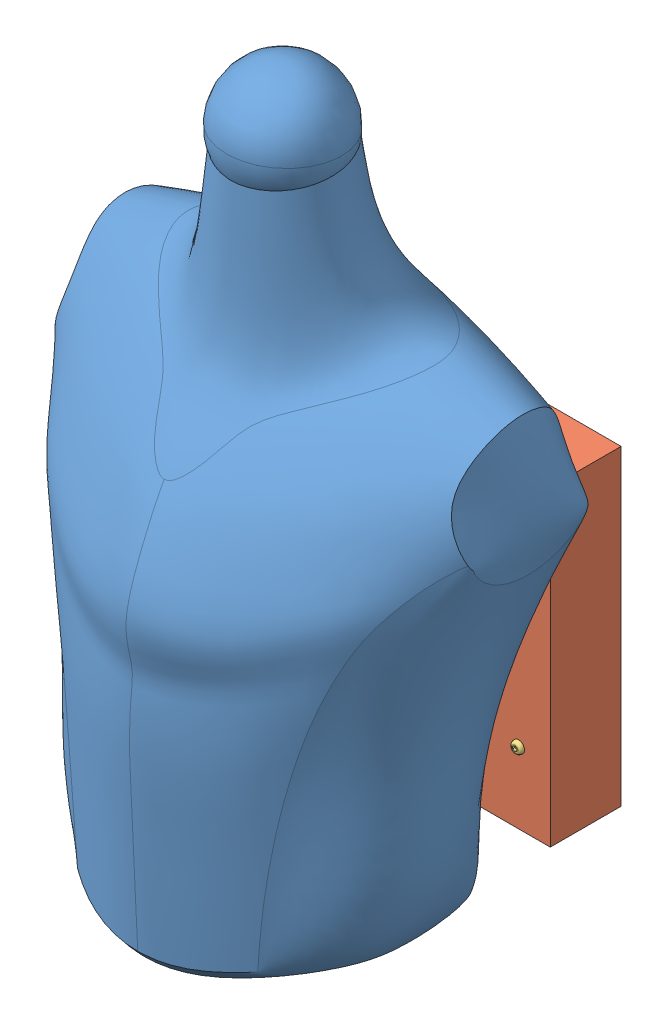
SolidWorks assembly ControlCircuitMount, configuration Default. Lengths in mm.
Overall size (402.84 950.58 367.01).
198 component instances, 41 part files, 56 mates.
Components (placement in the parent):
- AvgHumanBack-1: AvgHumanBack [Default] at origin size (402.84 950.58 279.6)
- ElectronicsBaseplate-1: ElectronicsBaseplate [Default] at (-35.085 1150.9976 -155.5) x (0 1 0) z (-1 0 0) size (224.52 47.62 183.13)
  - ControlPCB-1: ControlPCB [Default] at origin size (144.9 41.12 153.13)
    - MEGA2560+MotorShield-1: MEGA2560+MotorShield [Default] at origin size (108.32 25.5 53.3)
    - 1x2 Male Pin Header.step-1: 1x2 Male Pin Header.step [Default] at (-30.15 23.54 -23.8673) x (1 0 0) z (0 0 -1) size (5.08 13.54 2.5)
    - 1x6 Male Pin Header.step-1: 1x6 Male Pin Header.step [Default] at (-9.8 23.54 -23.8673) x (-1 0 0) z (0 0 1) size (15.24 13.54 2.5)
    - 1x5 Male Pin Header.step-1: 1x5 Male Pin Header.step [Default] at (-16.9 23.54 24.12) x (1 0 0) z (0 0 -1) size (12.71 13.54 2.5)
    - ADCPCB-1: ADCPCB [Default] at (-8.2861 23.54 0.0047) x (0.011416 0 0.999935) z (0 1 0) size (70.2 51.25 24.04)
      - 5x7PCBBoard.stp-1: 5x7PCBBoard.stp [Default] at origin size (70.2 50.2 1.66)
      - FemalePinHeader2By1.stp-1: FemalePinHeader2By1.stp [Default] at (-29.21 -21.59 1.54) x (0 1 0) z (0 0 1) size (5.08 2.54 11.7)
        - Female Pin Header 1x.stp-1: Female Pin Header 1x.stp [Default] at origin size (2.54 2.54 11.7)
        - Female Pin Header 1x.stp-2: Female Pin Header 1x.stp [Default] at (2.54 0 0) size (2.54 2.54 11.7)
      - FemalePinHeader2By1.stp-2: FemalePinHeader2By1.stp [Default] at (-29.21 -6.35 1.54) x (0 1 0) z (0 0 1) size (5.08 2.54 11.7)
        - Female Pin Header 1x.stp-1: Female Pin Header 1x.stp [Default] at origin size (2.54 2.54 11.7)
        - Female Pin Header 1x.stp-2: Female Pin Header 1x.stp [Default] at (2.54 0 0) size (2.54 2.54 11.7)
      - FemalePinHeader2By1.stp-3: FemalePinHeader2By1.stp [Default] at (-29.21 -19.05 1.54) x (0 1 0) z (0 0 1) size (5.08 2.54 11.7)
        - Female Pin Header 1x.stp-1: Female Pin Header 1x.stp [Default] at origin size (2.54 2.54 11.7)
        - Female Pin Header 1x.stp-2: Female Pin Header 1x.stp [Default] at (2.54 0 0) size (2.54 2.54 11.7)
      - FemalePinHeader2By1.stp-4: FemalePinHeader2By1.stp [Default] at (26.67 -21.59 1.54) x (0 1 0) z (0 0 1) size (5.08 2.54 11.7)
        - Female Pin Header 1x.stp-1: Female Pin Header 1x.stp [Default] at origin size (2.54 2.54 11.7)
        - Female Pin Header 1x.stp-2: Female Pin Header 1x.stp [Default] at (2.54 0 0) size (2.54 2.54 11.7)
      - FemalePinHeader2By1.stp-5: FemalePinHeader2By1.stp [Default] at (26.67 -19.05 1.54) x (0 1 0) z (0 0 1) size (5.08 2.54 11.7)
        - Female Pin Header 1x.stp-1: Female Pin Header 1x.stp [Default] at origin size (2.54 2.54 11.7)
        - Female Pin Header 1x.stp-2: Female Pin Header 1x.stp [Default] at (2.54 0 0) size (2.54 2.54 11.7)
      - FemalePinHeader10By1.stp-1: FemalePinHeader10By1.stp [Default] at (3.81 1.27 1.54) x (0 -1 0) z (0 0 1) size (25.4 2.54 11.7)
        - Female Pin Header 1x.stp-1: Female Pin Header 1x.stp [Default] at origin size (2.54 2.54 11.7)
        - Female Pin Header 1x.stp-2: Female Pin Header 1x.stp [Default] at (2.54 0 0) size (2.54 2.54 11.7)
        - Female Pin Header 1x.stp-3: Female Pin Header 1x.stp [Default] at (5.08 0 0) size (2.54 2.54 11.7)
        - Female Pin Header 1x.stp-4: Female Pin Header 1x.stp [Default] at (7.62 0 0) size (2.54 2.54 11.7)
        - Female Pin Header 1x.stp-5: Female Pin Header 1x.stp [Default] at (10.16 0 0) size (2.54 2.54 11.7)
        - Female Pin Header 1x.stp-6: Female Pin Header 1x.stp [Default] at (12.7 0 0) size (2.54 2.54 11.7)
        - Female Pin Header 1x.stp-7: Female Pin Header 1x.stp [Default] at (15.24 0 0) size (2.54 2.54 11.7)
        - Female Pin Header 1x.stp-8: Female Pin Header 1x.stp [Default] at (17.78 0 0) size (2.54 2.54 11.7)
        - Female Pin Header 1x.stp-9: Female Pin Header 1x.stp [Default] at (20.32 0 0) size (2.54 2.54 11.7)
        - Female Pin Header 1x.stp-10: Female Pin Header 1x.stp [Default] at (22.86 0 0) size (2.54 2.54 11.7)
      - FemalePinHeader6By1.stp-1: FemalePinHeader6By1.stp [Default] at (-13.97 21.59 1.54) x (0 -1 0) z (0 0 1) size (15.24 2.54 11.7)
        - Female Pin Header 1x.stp-1: Female Pin Header 1x.stp [Default] at origin size (2.54 2.54 11.7)
        - Female Pin Header 1x.stp-2: Female Pin Header 1x.stp [Default] at (2.54 0 0) size (2.54 2.54 11.7)
        - Female Pin Header 1x.stp-3: Female Pin Header 1x.stp [Default] at (5.08 0 0) size (2.54 2.54 11.7)
        - Female Pin Header 1x.stp-4: Female Pin Header 1x.stp [Default] at (7.62 0 0) size (2.54 2.54 11.7)
        - Female Pin Header 1x.stp-5: Female Pin Header 1x.stp [Default] at (10.16 0 0) size (2.54 2.54 11.7)
        - Female Pin Header 1x.stp-6: Female Pin Header 1x.stp [Default] at (12.7 0 0) size (2.54 2.54 11.7)
      - FemalePinHeader4By1.stp-1: FemalePinHeader4By1.stp [Default] at (11.44 19.05 1.54) x (0 -1 0) z (0 0 1) size (10.16 2.54 11.7)
        - Female Pin Header 1x.stp-1: Female Pin Header 1x.stp [Default] at origin size (2.54 2.54 11.7)
        - Female Pin Header 1x.stp-2: Female Pin Header 1x.stp [Default] at (2.54 0 0) size (2.54 2.54 11.7)
        - Female Pin Header 1x.stp-3: Female Pin Header 1x.stp [Default] at (5.08 0 0) size (2.54 2.54 11.7)
        - Female Pin Header 1x.stp-4: Female Pin Header 1x.stp [Default] at (7.62 0 0) size (2.54 2.54 11.7)
      - ADS1115+PinHeader.step-1: ADS1115+PinHeader.step [Default] at (144.065 -99.14 12.63) x (-1 0 0) z (0 0 1) size (17.14 27.94 11.54)
        - R_0805_2012Metric.step-1: R_0805_2012Metric.step [Default] at (149.225 -80.01 1.65) size (2 1.2 0.45)
          - SOLID.step-1: SOLID.step [Default] at origin size (2 1.2 0.45)
        - R_0805_2012Metric.step-2: R_0805_2012Metric.step [Default] at (149.225 -77.47 1.65) size (2 1.2 0.45)
          - SOLID.step-1: SOLID.step [Default] at origin size (2 1.2 0.45)
        - C_0603_1608Metric.step-1: C_0603_1608Metric.step [Default] at (150.495 -96.52 1.65) x (0 1 0) z (0 0 1) size (1.6 0.8 0.8)
          - SOLID-0.step-1: SOLID-0.step [Default] at origin size (1.6 0.8 0.8)
        - TSSOP-10_3x3mm_P0.5mm.step-1: TSSOP-10_3x3mm_P0.5mm.step [Default] at (147.32 -96.52 1.65) x (0 -1 0) z (0 0 1) size (4.9 3 1)
          - SOLID-1.step-1: SOLID-1.step [Default] at origin size (4.9 3 1)
        - PinHeader_1x10_P2.54mm_Vertical.step-1: PinHeader_1x10_P2.54mm_Vertical.step [Default] at (140.335 -77.47 -0.05) x (-1 0 0) z (0 0 -1) size (2.54 25.4 11.54)
          - SOLID-2.step-1: SOLID-2.step [Default] at origin size (2.54 25.4 11.54)
        - C_0603_1608Metric.step-2: C_0603_1608Metric.step [Default] at (146.05 -78.74 1.65) x (0 1 0) z (0 0 1) size (1.6 0.8 0.8)
          - SOLID-0.step-1: SOLID-0.step [Default] at origin size (1.6 0.8 0.8)
        - R_0402_1005Metric.step-1: R_0402_1005Metric.step [Default] at (149.225 -85.09 1.65) x (-1 0 0) z (0 0 1) size (1 0.5 0.35)
          - SOLID-3.step-1: SOLID-3.step [Default] at origin size (1 0.5 0.35)
        - R_0402_1005Metric.step-2: R_0402_1005Metric.step [Default] at (149.225 -82.55 1.65) x (-1 0 0) z (0 0 1) size (1 0.5 0.35)
          - SOLID-3.step-1: SOLID-3.step [Default] at origin size (1 0.5 0.35)
        - R_0402_1005Metric.step-3: R_0402_1005Metric.step [Default] at (149.225 -87.63 1.65) size (1 0.5 0.35)
          - SOLID-3.step-1: SOLID-3.step [Default] at origin size (1 0.5 0.35)
        - R_0402_1005Metric.step-4: R_0402_1005Metric.step [Default] at (149.225 -90.17 1.65) x (-1 0 0) z (0 0 1) size (1 0.5 0.35)
          - SOLID-3.step-1: SOLID-3.step [Default] at origin size (1 0.5 0.35)
        - COMPOUND.step-1: COMPOUND.step [Default] at origin size (17.14 27.94 1.6)
      - 1x4 Male Pin Header.step-1: 1x4 Male Pin Header.step [Default] at (11.52 11.51 12.58) x (0 1 0) z (-1 0 0) size (10.17 13.54 2.5)
      - 1x6 Male Pin Header.step-1: 1x6 Male Pin Header.step [Default] at (-13.89 8.97 12.58) x (0 1 0) z (-1 0 0) size (15.24 13.54 2.5)
      - HX711.STEP-1: HX711.STEP [Default] at (-17.9207 5.1545 12.58) size (34 21 1.97)
        - HX711_SOP16_Valor predeterminado.STEP-1: HX711_SOP16_Valor predeterminado.STEP [Default] at (16.3915 14.4374 -9.5535) size (6.7 10 1.56)
          - base_HX711_Valor predeterminado.STEP-1: base_HX711_Valor predeterminado.STEP [Default] at (0.6189 -0.8581 10) size (4.4 10 1.52)
          - pino_HX711_Valor predeterminado.STEP-1: pino_HX711_Valor predeterminado.STEP [Default] at (-2.7311 3.5869 10.04) x (0 -1 0) z (-1 0 0) size (0.4 0.86 1.3)
          - pino_HX711_Valor predeterminado.STEP-2: pino_HX711_Valor predeterminado.STEP [Default] at (-2.7311 2.3169 10.04) x (0 -1 0) z (-1 0 0) size (0.4 0.86 1.3)
          - pino_HX711_Valor predeterminado.STEP-3: pino_HX711_Valor predeterminado.STEP [Default] at (-2.7311 1.0469 10.04) x (0 -1 0) z (-1 0 0) size (0.4 0.86 1.3)
          - pino_HX711_Valor predeterminado.STEP-4: pino_HX711_Valor predeterminado.STEP [Default] at (-2.7311 -0.2231 10.04) x (0 -1 0) z (-1 0 0) size (0.4 0.86 1.3)
          - pino_HX711_Valor predeterminado.STEP-5: pino_HX711_Valor predeterminado.STEP [Default] at (-2.7311 -1.4931 10.04) x (0 -1 0) z (-1 0 0) size (0.4 0.86 1.3)
          - pino_HX711_Valor predeterminado.STEP-6: pino_HX711_Valor predeterminado.STEP [Default] at (-2.7311 -2.7631 10.04) x (0 -1 0) z (-1 0 0) size (0.4 0.86 1.3)
          - pino_HX711_Valor predeterminado.STEP-7: pino_HX711_Valor predeterminado.STEP [Default] at (-2.7311 -4.0331 10.04) x (0 -1 0) z (-1 0 0) size (0.4 0.86 1.3)
          - pino_HX711_Valor predeterminado.STEP-8: pino_HX711_Valor predeterminado.STEP [Default] at (-2.7311 -5.3031 10.04) x (0 -1 0) z (-1 0 0) size (0.4 0.86 1.3)
          - pino_HX711_Valor predeterminado.STEP-9: pino_HX711_Valor predeterminado.STEP [Default] at (3.9689 3.5869 10.04) x (0 1 0) z (1 0 0) size (0.4 0.86 1.3)
          - pino_HX711_Valor predeterminado.STEP-10: pino_HX711_Valor predeterminado.STEP [Default] at (3.9689 2.3169 10.04) x (0 1 0) z (1 0 0) size (0.4 0.86 1.3)
          - pino_HX711_Valor predeterminado.STEP-11: pino_HX711_Valor predeterminado.STEP [Default] at (3.9689 1.0469 10.04) x (0 1 0) z (1 0 0) size (0.4 0.86 1.3)
          - pino_HX711_Valor predeterminado.STEP-12: pino_HX711_Valor predeterminado.STEP [Default] at (3.9689 -0.2231 10.04) x (0 1 0) z (1 0 0) size (0.4 0.86 1.3)
          - pino_HX711_Valor predeterminado.STEP-13: pino_HX711_Valor predeterminado.STEP [Default] at (3.9689 -1.4931 10.04) x (0 1 0) z (1 0 0) size (0.4 0.86 1.3)
          - pino_HX711_Valor predeterminado.STEP-14: pino_HX711_Valor predeterminado.STEP [Default] at (3.9689 -2.7631 10.04) x (0 1 0) z (1 0 0) size (0.4 0.86 1.3)
          - pino_HX711_Valor predeterminado.STEP-15: pino_HX711_Valor predeterminado.STEP [Default] at (3.9689 -4.0331 10.04) x (0 1 0) z (1 0 0) size (0.4 0.86 1.3)
          - pino_HX711_Valor predeterminado.STEP-16: pino_HX711_Valor predeterminado.STEP [Default] at (3.9689 -5.3031 10.04) x (0 1 0) z (1 0 0) size (0.4 0.86 1.3)
        - SOT23_Valor predeterminado.STEP-1: SOT23_Valor predeterminado.STEP [Default] at (9.1544 19.1355 -2.4535) x (-1 0 0) z (0 0 1) size (2.3 2.9 1.03)
          - TRANSISTOR_SOT23_Valor predeterminado.STEP-1: TRANSISTOR_SOT23_Valor predeterminado.STEP [Default] at (0.0204 0.1428 2.9) size (1.3 2.9 1)
          - PINO_SOT23_Valor predeterminado.STEP-1: PINO_SOT23_Valor predeterminado.STEP [Default] at (-1.1296 1.0928 2.94) x (0 -1 0) z (-1 0 0) size (0.4 0.61 0.65)
          - PINO_SOT23_Valor predeterminado.STEP-2: PINO_SOT23_Valor predeterminado.STEP [Default] at (-1.1296 -0.8072 2.94) x (0 -1 0) z (-1 0 0) size (0.4 0.61 0.65)
          - PINO_SOT23_Valor predeterminado.STEP-3: PINO_SOT23_Valor predeterminado.STEP [Default] at (1.1704 0.1428 2.94) x (0 1 0) z (1 0 0) size (0.4 0.61 0.65)
        - placa_Valor predeterminado.STEP-1: placa_Valor predeterminado.STEP [Default] at origin size (34 21 0.41)
        - RESISTOR_SMD_122_Valor predeterminado.STEP-1: RESISTOR_SMD_122_Valor predeterminado.STEP [Default] at (7.557 7.2289 0.4215) x (0 1 0) z (-1 0 0) size (2 0.82 1.27)
        - RESISTOR_SMD_122_Valor predeterminado.STEP-2: RESISTOR_SMD_122_Valor predeterminado.STEP [Default] at (26.4556 7.0756 0.4215) x (0 1 0) z (-1 0 0) size (2 0.82 1.27)
        - RESISTOR_SMD_822_Valor predeterminado.STEP-1: RESISTOR_SMD_822_Valor predeterminado.STEP [Default] at (8.9272 12.9039 0.4215) x (-1 0 0) z (0 -1 0) size (2 0.82 1.27)
        - RESISTOR_SMD_203_Valor predeterminado.STEP-1: RESISTOR_SMD_203_Valor predeterminado.STEP [Default] at (8.9446 15.4759 0.4215) x (-1 0 0) z (0 -1 0) size (2 0.82 1.27)
        - CAPACITOR_805_Valor predeterminado.STEP-1: CAPACITOR_805_Valor predeterminado.STEP [Default] at (14.517 4.7561 0.4215) x (1 0 0) z (0 1 0) size (2 0.8 1.27)
        - CAPACITOR_805_Valor predeterminado.STEP-2: CAPACITOR_805_Valor predeterminado.STEP [Default] at (24.8147 18.1011 0.4215) x (1 0 0) z (0 1 0) size (2 0.8 1.27)
        - CAPACITOR_805_Valor predeterminado.STEP-3: CAPACITOR_805_Valor predeterminado.STEP [Default] at (19.4533 4.8571 0.4215) x (1 0 0) z (0 1 0) size (2 0.8 1.27)
        - CAPACITOR_805_Valor predeterminado.STEP-4: CAPACITOR_805_Valor predeterminado.STEP [Default] at (23.7861 6.9684 0.4215) x (0 -1 0) z (1 0 0) size (2 0.8 1.27)
        - CAPACITOR_805_Valor predeterminado.STEP-5: CAPACITOR_805_Valor predeterminado.STEP [Default] at (10.279 7.2922 0.4215) x (0 -1 0) z (1 0 0) size (2 0.8 1.27)
      - 1x2 Male Pin Header.step-1: 1x2 Male Pin Header.step [Default] at (-29.29 -19.13 10.04) x (0 -1 0) z (-1 0 0) size (5.08 13.54 2.5) (hidden)
      - 1x2 Male Pin Header.step-2: 1x2 Male Pin Header.step [Default] at (-29.29 -3.89 10.04) x (0 -1 0) z (-1 0 0) size (5.08 13.54 2.5) (hidden)
      - 1x2 Male Pin Header.step-3: 1x2 Male Pin Header.step [Default] at (26.59 -16.59 10.04) x (0 -1 0) z (-1 0 0) size (5.08 13.54 2.5) (hidden)
      - 5mm2PTerminalBlock-1: 5mm2PTerminalBlock [Default] at (-25.19 24.09 1.54) x (0 -1 0) z (0 0 1) size (10.6 7.6 15)
      - 5mm2PTerminalBlock-2: 5mm2PTerminalBlock [Default] at (-25.19 13.89 1.54) x (0 -1 0) z (0 0 1) size (10.6 7.6 15)
      - 5mm2PTerminalBlock-3: 5mm2PTerminalBlock [Default] at (3.69 25.19 1.54) x (-1 0 0) z (0 0 1) size (10.6 7.6 15)
      - 5mm2PTerminalBlock-4: 5mm2PTerminalBlock [Default] at (15.04 -6.23 1.54) x (0 1 0) z (0 0 1) size (10.6 7.6 15)
    - BLEShuntPCB-1: BLEShuntPCB [Default] at (-12.5947 21 -49.5125) x (-1 0 0) z (0 -1 0) size (73.24 30.62 25.87)
      - 3x7PerfBoard-1: 3x7PerfBoard [Default] at origin size (70.1 30.1 1.65)
      - 5mm2PTerminalBlock-1: 5mm2PTerminalBlock [Default] at (-19.17 15.03 1.55) x (-1 0 0) z (0 0 1) size (10.6 7.6 15)
      - FemalePinHeader8By1.stp-1: FemalePinHeader8By1.stp [Default] at (-16.51 6.35 1.55) x (0 -1 0) z (0 0 1) size (20.32 2.54 11.7)
        - Female Pin Header 1x.stp-1: Female Pin Header 1x.stp [Default] at origin size (2.54 2.54 11.7)
        - Female Pin Header 1x.stp-2: Female Pin Header 1x.stp [Default] at (2.54 0 0) size (2.54 2.54 11.7)
        - Female Pin Header 1x.stp-3: Female Pin Header 1x.stp [Default] at (5.08 0 0) size (2.54 2.54 11.7)
        - Female Pin Header 1x.stp-4: Female Pin Header 1x.stp [Default] at (7.62 0 0) size (2.54 2.54 11.7)
        - Female Pin Header 1x.stp-5: Female Pin Header 1x.stp [Default] at (10.16 0 0) size (2.54 2.54 11.7)
        - Female Pin Header 1x.stp-6: Female Pin Header 1x.stp [Default] at (12.7 0 0) size (2.54 2.54 11.7)
        - Female Pin Header 1x.stp-7: Female Pin Header 1x.stp [Default] at (15.24 0 0) size (2.54 2.54 11.7)
        - Female Pin Header 1x.stp-8: Female Pin Header 1x.stp [Default] at (17.78 0 0) size (2.54 2.54 11.7)
      - 1x8 Male Pin Header.step-1: 1x8 Male Pin Header.step [Default] at (-16.59 6.27 12.59) x (0 -1 0) z (1 0 0) size (20.32 13.54 2.5)
      - BLEFriend.stp-1: BLEFriend.stp [Default] at (-19.31 8.128 12.59) x (0 -1 0) z (0 0 1) size (21.35 31.87 4.78)
      - 5mm2PTerminalBlock-2: 5mm2PTerminalBlock [Default] at (24.01 15.03 1.55) x (-1 0 0) z (0 0 1) size (10.6 7.6 15)
      - 5mm2PTerminalBlock-5: 5mm2PTerminalBlock [Default] at (14.1 -15.03 1.55) size (10.6 7.6 15)
      - FemalePinHeader2By1-1: FemalePinHeader2By1 [Default] at (-29.21 -8.89 0) x (0 -1 0) z (0 0 -1) size (5.08 2.54 11.7)
      - FemalePinHeader2By1-2: FemalePinHeader2By1 [Default] at (-29.21 6.35 0) x (0 -1 0) z (0 0 -1) size (5.08 2.54 11.7)
      - FemalePinHeader2By1-3: FemalePinHeader2By1 [Default] at (26.67 -6.35 0) x (0 -1 0) z (0 0 -1) size (5.08 2.54 11.7)
      - ShuntResistor-1: ShuntResistor [Default<As Machined>] at (18.3281 0.2483 1.55) x (0.946299 -0.323291 0) z (-0.323291 -0.946299 0) size (35 9.71 20.4)
    - RelayPCB-1: RelayPCB [Default] at (46.44 18.5 -16.8) x (0 0 -1) z (1 0 0) size (51 20.5 20)
    - ThermistorPCB-1: ThermistorPCB [Default] at (53.61 18 26.48) x (0 0 -1) z (1 0 0) size (30 20 70)
    - RelayPCB-2: RelayPCB [Default] at (109.78 0 -53.12) size (55.5 16.25 117.54)
      - 4-Port Relay-1: 4-Port Relay [Default] at origin size (55.5 16.25 75.54)
      - 2-Port Relay-1: 2-Port Relay [Default] at (2.75 0 60.27) size (50 16.25 39)
    - LM2596-BuckConverter-1: LM2596-BuckConverter [Default] at (-16.99 0 -92.15) x (-1 0 0) z (0 1 0) size (65 39 13)
    - LM2596-BuckConverter-2: LM2596-BuckConverter [Default] at (48.77 0 -79.15) x (0 0 -1) z (0 1 0) size (65 39 13)
  - Baseplate^ElectronicsBaseplate-1: Baseplate^ElectronicsBaseplate [Default] at (30 0 0) size (224.52 14.95 183.13) (virtual)
  - M3x8-1: M3x8 [Default] at (-35.49 -5.5 24.11) x (1 0 0) z (0 -1 0) size (5.5 5.5 11)
  - M3x8-2: M3x8 [Default] at (46.98 -5.5 24.11) x (1 0 0) z (0 -1 0) size (5.5 5.5 11)
  - M3x8-3: M3x8 [Default] at (40.62 -5.5 -24.11) x (1 0 0) z (0 -1 0) size (5.5 5.5 11)
  - M3x8-4: M3x8 [Default] at (-34.26 -5.5 -24.11) x (1 0 0) z (0 -1 0) size (5.5 5.5 11)
  - M3x8-5: M3x8 [Default] at (-45.99 -5.5 -76.15) x (1 0 0) z (0 -1 0) size (5.5 5.5 11)
  - M3x8-6: M3x8 [Default] at (12.01 -5.5 -76.15) x (1 0 0) z (0 -1 0) size (5.5 5.5 11)
  - M3x8-7: M3x8 [Default] at (-45.99 -5.5 -108.15) x (1 0 0) z (0 -1 0) size (5.5 5.5 11)
  - M3x8-8: M3x8 [Default] at (12.01 -5.5 -108.15) x (1 0 0) z (0 -1 0) size (5.5 5.5 11)
  - M3x8-9: M3x8 [Default] at (32.77 -5.5 -50.15) x (1 0 0) z (0 -1 0) size (5.5 5.5 11)
  - M3x8-10: M3x8 [Default] at (64.77 -5.5 -50.15) x (1 0 0) z (0 -1 0) size (5.5 5.5 11)
  - M3x8-11: M3x8 [Default] at (32.77 -5.5 -108.15) x (1 0 0) z (0 -1 0) size (5.5 5.5 11)
  - M3x8-12: M3x8 [Default] at (64.77 -5.5 -108.15) x (1 0 0) z (0 -1 0) size (5.5 5.5 11)
  - M3x8-13: M3x8 [Default] at (85.655 -5.5 -87.245) x (1 0 0) z (0 -1 0) size (5.5 5.5 11)
  - M3x8-14: M3x8 [Default] at (133.905 -5.5 -87.245) x (1 0 0) z (0 -1 0) size (5.5 5.5 11)
  - M3x8-15: M3x8 [Default] at (133.905 -5.5 -18.995) x (1 0 0) z (0 -1 0) size (5.5 5.5 11)
  - M3x8-16: M3x8 [Default] at (85.655 -5.5 -18.995) x (1 0 0) z (0 -1 0) size (5.5 5.5 11)
  - M3x8-17: M3x8 [Default] at (89.905 -5.5 -9.6) x (1 0 0) z (0 -1 0) size (5.5 5.5 11)
  - M3x8-18: M3x8 [Default] at (135.155 -5.5 -9.6) x (1 0 0) z (0 -1 0) size (5.5 5.5 11)
  - M3x8-19: M3x8 [Default] at (89.905 -5.5 23.9) x (1 0 0) z (0 -1 0) size (5.5 5.5 11)
  - M3x8-20: M3x8 [Default] at (135.155 -5.5 23.9) x (1 0 0) z (0 -1 0) size (5.5 5.5 11)
  - M3x8-22: M3x8 [Default] at (16.53 -5.5 -8.88) x (1 0 0) z (0 -1 0) size (5.5 5.5 11)
  - M3x8-23: M3x8 [Default] at (16.53 -5.5 19.03) x (1 0 0) z (0 -1 0) size (5.5 5.5 11)
  - M3Nut-1: M3Nut [Default] at (32.77 1.5 -108.15) size (6 2.34 5.2)
  - M3Nut-2: M3Nut [Default] at (64.77 1.5 -108.15) size (6 2.34 5.2)
  - M3Nut-3: M3Nut [Default] at (32.77 1.5 -50.15) size (6 2.34 5.2)
  - M3Nut-4: M3Nut [Default] at (64.77 1.5 -50.15) size (6 2.34 5.2)
  - M3Nut-7: M3Nut [Default] at (12.01 1.5 -108.15) size (6 2.34 5.2)
  - M3Nut-8: M3Nut [Default] at (-45.99 1.5 -108.15) size (6 2.34 5.2)
  - M3Nut-9: M3Nut [Default] at (-45.99 1.5 -76.15) size (6 2.34 5.2)
  - M3Nut-10: M3Nut [Default] at (12.01 1.5 -76.15) size (6 2.34 5.2)
  - M3Nut-11: M3Nut [Default] at (-34.26 1.5 -24.11) size (6 2.34 5.2)
  - M3Nut-12: M3Nut [Default] at (-35.49 1.5 24.11) size (6 2.34 5.2)
  - M3Nut-13: M3Nut [Default] at (16.53 1.5 19.03) size (6 2.34 5.2)
  - M3Nut-14: M3Nut [Default] at (16.53 1.5 -8.88) size (6 2.34 5.2)
  - M3Nut-17: M3Nut [Default] at (85.655 1.75 -87.245) size (6 2.34 5.2)
  - M3Nut-19: M3Nut [Default] at (133.905 1.75 -87.245) size (6 2.34 5.2)
  - M3Nut-20: M3Nut [Default] at (133.905 1.75 -18.995) size (6 2.34 5.2)
  - M3Nut-21: M3Nut [Default] at (85.655 1.75 -18.995) size (6 2.34 5.2)
  - M3Nut-22: M3Nut [Default] at (89.905 1.75 -9.6) size (6 2.34 5.2)
  - M3Nut-23: M3Nut [Default] at (135.155 1.75 -9.6) size (6 2.34 5.2)
  - M3Nut-24: M3Nut [Default] at (135.155 1.75 23.9) size (6 2.34 5.2)
  - M3Nut-25: M3Nut [Default] at (89.905 1.75 23.9) size (6 2.34 5.2)
- PlasticBox-1: PlasticBox [Default] at (11.048 1111.6872 -147) size (215.9 279.4 63.5)
- M6x12_Buttonhead-1: M6x12_Buttonhead [Default] at (83.565 1203.7676 -144) x (0.866025 0.5 0) z (0 0 1) size (10.53 10.53 15.3)
- M6x12_Buttonhead-2: M6x12_Buttonhead [Default] at (49.565 1296.0276 -144) x (0.866025 0.5 0) z (0 0 1) size (10.53 10.53 15.3)
- M6x12_Buttonhead-3: M6x12_Buttonhead [Default] at (79.565 1093.5076 -144) x (0.866025 0.5 0) z (0 0 1) size (10.53 10.53 15.3)
- M6x12_Buttonhead-4: M6x12_Buttonhead [Default] at (-79.565 1296.0276 -144) x (0.866025 0.5 0) z (0 0 1) size (10.53 10.53 15.3)
- M6x12_Buttonhead-5: M6x12_Buttonhead [Default] at (-79.565 1203.7676 -144) x (0.866025 0.5 0) z (0 0 1) size (10.53 10.53 15.3)
- M6x12_Buttonhead-6: M6x12_Buttonhead [Default] at (-79.565 1093.5076 -144) x (0.866025 0.5 0) z (0 0 1) size (10.53 10.53 15.3)
- M6Nut-1: M6Nut [Default] at (79.565 1093.5076 -153) x (0 1 0) z (-1 0 0) size (11.08 5.03 10.65)
- M6Nut-2: M6Nut [Default] at (83.565 1203.7676 -153) x (0 1 0) z (-1 0 0) size (11.08 5.03 10.65)
- M6Nut-3: M6Nut [Default] at (49.565 1296.0276 -153) x (0 1 0) z (-1 0 0) size (11.08 5.03 10.65)
- M6Nut-4: M6Nut [Default] at (-79.565 1296.0276 -153) x (0 1 0) z (-1 0 0) size (11.08 5.03 10.65)
- M6Nut-5: M6Nut [Default] at (-79.565 1203.7676 -153) x (0 1 0) z (-1 0 0) size (11.08 5.03 10.65)
- M6Nut-6: M6Nut [Default] at (-79.565 1093.5076 -153) x (0 1 0) z (-1 0 0) size (11.08 5.03 10.65)
- BatteryMount-1: BatteryMount [Default] at (42.2 1067.9476 -164.44) x (1 0 0) z (0 1 0) size (166.9 85.99 60.11)
  - BatteryPack-1: BatteryPack [Default] at origin size (166.9 85.99 36.23)
  - BatteryPack-2: BatteryPack [Default] at (0 0 -23.88) size (166.9 85.99 36.23)
Mates (geometry in assembly coordinates):
- Coincident1: coincident aligned: plane of AvgHumanBack-1 through (0 0 0) normal (0 0 1)
- Coincident2: coincident aligned: plane of AvgHumanBack-1 through (0 0 0) normal (0 1 0)
- Coincident3: coincident aligned: plane of AvgHumanBack-1 through (0 0 0) normal (1 0 0)
- Parallel1: parallel aligned: plane of ElectronicsBaseplate-1/Baseplate^ElectronicsBaseplate-1 through (-35.085 1180.9976 -150) normal (0 0 1)
- Coincident6: coincident aligned: plane of ElectronicsBaseplate-1/Baseplate^ElectronicsBaseplate-1 through (-35.085 1180.9976 -150) normal (0 0 1)
- Tangent1: tangent: face of ?; plane of assembly through (0 0 -150) normal (0 0 1)
- Symmetric2: symmetric aligned: plane of BatteryPack-1 through (66.3 1055.1849 -161.49) normal (1 0 0); plane of BatteryPack-1 through (-66.3 1055.1849 -161.49) normal (-1 0 0)
- InPlace1: in place: plane of AvgHumanBack-1 through (0 0 0) normal (0 0 1); moOrthogonalPlaneRef_w of AvgHumanBack-1 through (0 0 0) normal (0 1 0); plane of AvgHumanBack-1 through (0 0 0) normal (1 0 0); unknown of AvgHumanBack-1
- Coincident10: coincident aligned: 
- Coincident11: coincident aligned: plane of Part1^ControlCircuitMount-1 through (0 0 0) normal (0 1 0)
- Coincident12: coincident anti-aligned: plane of Part1^ControlCircuitMount-1 through (0 0 0) normal (1 0 0)
- Symmetric5: symmetric aligned: plane of Tote^ControlCircuitMount-1 through (104.95 1032.6276 -207.5) normal (-1 0 0); plane of Tote^ControlCircuitMount-1 through (-104.95 1306.0276 -207.5) normal (1 0 0)
- Coincident26: coincident anti-aligned: plane of ElectronicsBaseplate-1/M3x8-3 through (-10.975 1191.6176 -147) normal (0 0 1); plane of Tote^ControlCircuitMount-1 through (11.048 1111.6872 -147) normal (0 0 -1)
- Coincident17: coincident: point of AvgHumanBack-1; plane of Tote^ControlCircuitMount-1 through (-107.95 1029.6276 -144) normal (0 -1 0)
- Coincident18: coincident anti-aligned: plane of Tote^ControlCircuitMount-1 through (11.048 1111.6872 -144) normal (0 0 1); plane of M6x12_Buttonhead-1 through (83.565 1203.7676 -144) normal (0 0 -1)
- Parallel3: parallel anti-aligned: plane of Tote^ControlCircuitMount-1 through (-107.95 1309.0276 -144) normal (-1 0 0); plane of M6x12_Buttonhead-1 through (81.5645 1204.9226 -142.78) normal (1 0 0)
- Concentric1: concentric aligned: circle of Tote^ControlCircuitMount-1; circle of M6x12_Buttonhead-1
- Coincident20: coincident anti-aligned: plane of Tote^ControlCircuitMount-1 through (11.048 1111.6872 -144) normal (0 0 1); plane of M6x12_Buttonhead-2 through (49.565 1296.0276 -144) normal (0 0 -1)
- Parallel4: parallel anti-aligned: plane of Tote^ControlCircuitMount-1 through (-107.95 1309.0276 -144) normal (-1 0 0); plane of M6x12_Buttonhead-2 through (47.5645 1297.1826 -142.78) normal (1 0 0)
- Concentric2: concentric aligned: circle of Tote^ControlCircuitMount-1; circle of M6x12_Buttonhead-2
- Coincident21: coincident anti-aligned: plane of Tote^ControlCircuitMount-1 through (11.048 1111.6872 -144) normal (0 0 1); plane of M6x12_Buttonhead-3 through (79.565 1093.5076 -144) normal (0 0 -1)
- Parallel5: parallel anti-aligned: plane of Tote^ControlCircuitMount-1 through (-107.95 1309.0276 -144) normal (-1 0 0); plane of M6x12_Buttonhead-3 through (77.5645 1094.6626 -142.78) normal (1 0 0)
- Concentric3: concentric aligned: circle of Tote^ControlCircuitMount-1; circle of M6x12_Buttonhead-3
- Coincident22: coincident anti-aligned: plane of Tote^ControlCircuitMount-1 through (11.048 1111.6872 -144) normal (0 0 1); plane of M6x12_Buttonhead-4 through (-79.565 1296.0276 -144) normal (0 0 -1)
- Parallel6: parallel anti-aligned: plane of Tote^ControlCircuitMount-1 through (-107.95 1309.0276 -144) normal (-1 0 0); plane of M6x12_Buttonhead-4 through (-81.5655 1297.1826 -142.78) normal (1 0 0)
- Concentric4: concentric aligned: circle of Tote^ControlCircuitMount-1; circle of M6x12_Buttonhead-4
- Coincident23: coincident anti-aligned: plane of Tote^ControlCircuitMount-1 through (11.048 1111.6872 -144) normal (0 0 1); plane of M6x12_Buttonhead-5 through (-79.565 1203.7676 -144) normal (0 0 -1)
- Parallel7: parallel anti-aligned: plane of Tote^ControlCircuitMount-1 through (-107.95 1309.0276 -144) normal (-1 0 0); plane of M6x12_Buttonhead-5 through (-81.5655 1204.9226 -142.78) normal (1 0 0)
- Concentric5: concentric aligned: circle of Tote^ControlCircuitMount-1; circle of M6x12_Buttonhead-5
- Coincident24: coincident anti-aligned: plane of Tote^ControlCircuitMount-1 through (11.048 1111.6872 -144) normal (0 0 1); plane of M6x12_Buttonhead-6 through (-79.565 1093.5076 -144) normal (0 0 -1)
- Parallel8: parallel anti-aligned: plane of Tote^ControlCircuitMount-1 through (-107.95 1309.0276 -144) normal (-1 0 0); plane of M6x12_Buttonhead-6 through (-81.5655 1094.6626 -142.78) normal (1 0 0)
- Parallel10: parallel anti-aligned: plane of Tote^ControlCircuitMount-1 through (104.95 1032.6276 -207.5) normal (-1 0 0); plane of M6Nut-1 through (84.49 1096.351 -157.85) normal (1 0 0)
- Concentric7: concentric aligned: circle of M6x12_Buttonhead-3; circle of M6Nut-1
- Parallel11: parallel anti-aligned: plane of Tote^ControlCircuitMount-1 through (104.95 1032.6276 -207.5) normal (-1 0 0); plane of M6Nut-2 through (88.49 1206.611 -157.85) normal (1 0 0)
- Concentric8: concentric aligned: circle of M6x12_Buttonhead-1; circle of M6Nut-2
- Parallel12: parallel anti-aligned: plane of Tote^ControlCircuitMount-1 through (104.95 1032.6276 -207.5) normal (-1 0 0); plane of M6Nut-3 through (54.49 1298.871 -157.85) normal (1 0 0)
- Concentric9: concentric aligned: circle of M6x12_Buttonhead-2; circle of M6Nut-3
- Parallel13: parallel anti-aligned: plane of Tote^ControlCircuitMount-1 through (104.95 1032.6276 -207.5) normal (-1 0 0); plane of M6Nut-4 through (-74.64 1298.871 -157.85) normal (1 0 0)
- Concentric10: concentric aligned: circle of M6x12_Buttonhead-4; circle of M6Nut-4
- Parallel14: parallel anti-aligned: plane of Tote^ControlCircuitMount-1 through (104.95 1032.6276 -207.5) normal (-1 0 0); plane of M6Nut-5 through (-74.64 1206.611 -157.85) normal (1 0 0)
- Concentric11: concentric aligned: circle of M6x12_Buttonhead-5; circle of M6Nut-5
- Parallel15: parallel anti-aligned: plane of Tote^ControlCircuitMount-1 through (104.95 1032.6276 -207.5) normal (-1 0 0); plane of M6Nut-6 through (-74.64 1096.351 -157.85) normal (1 0 0)
- Concentric12: concentric aligned: circle of M6x12_Buttonhead-6; circle of M6Nut-6
- Parallel16: parallel anti-aligned: plane of ElectronicsBaseplate-1/Baseplate^ElectronicsBaseplate-1 through (-91.565 1081.5076 -150) normal (0 -1 0); plane of Tote^ControlCircuitMount-1 through (-104.95 1032.6276 -207.5) normal (0 1 0)
- Symmetric6: symmetric aligned: plane of ElectronicsBaseplate-1/Baseplate^ElectronicsBaseplate-1 through (-91.565 1306.0276 -150) normal (-1 0 0); plane of ElectronicsBaseplate-1/Baseplate^ElectronicsBaseplate-1 through (91.565 1081.5076 -150) normal (1 0 0)
- Coincident36: coincident anti-aligned: plane of ElectronicsBaseplate-1/Baseplate^ElectronicsBaseplate-1 through (61.565 1306.0276 -150) normal (0 1 0); plane of Tote^ControlCircuitMount-1 through (104.95 1306.0276 -207.5) normal (0 -1 0)
- Concentric13: concentric anti-aligned: circle of ElectronicsBaseplate-1/Baseplate^ElectronicsBaseplate-1; circle of M6x12_Buttonhead-6
- Coincident37: coincident anti-aligned: plane of ElectronicsBaseplate-1/Baseplate^ElectronicsBaseplate-1 through (-35.085 1180.9976 -153) normal (0 0 -1); plane of M6Nut-1 through (79.565 1093.5076 -153) normal (0 0 1)
- Coincident38: coincident anti-aligned: plane of ElectronicsBaseplate-1/Baseplate^ElectronicsBaseplate-1 through (-35.085 1180.9976 -153) normal (0 0 -1); plane of M6Nut-6 through (-79.565 1093.5076 -153) normal (0 0 1)
- Coincident39: coincident anti-aligned: plane of ElectronicsBaseplate-1/Baseplate^ElectronicsBaseplate-1 through (-35.085 1180.9976 -153) normal (0 0 -1); plane of M6Nut-5 through (-79.565 1203.7676 -153) normal (0 0 1)
- Coincident40: coincident anti-aligned: plane of ElectronicsBaseplate-1/Baseplate^ElectronicsBaseplate-1 through (-35.085 1180.9976 -153) normal (0 0 -1); plane of M6Nut-2 through (83.565 1203.7676 -153) normal (0 0 1)
- Coincident41: coincident anti-aligned: plane of ElectronicsBaseplate-1/Baseplate^ElectronicsBaseplate-1 through (-35.085 1180.9976 -153) normal (0 0 -1); plane of M6Nut-4 through (-79.565 1296.0276 -153) normal (0 0 1)
- Coincident42: coincident anti-aligned: plane of ElectronicsBaseplate-1/Baseplate^ElectronicsBaseplate-1 through (-35.085 1180.9976 -153) normal (0 0 -1); plane of M6Nut-3 through (49.565 1296.0276 -153) normal (0 0 1)
- Symmetric7: symmetric aligned: plane of BatteryMount-1/BatteryPack-2 through (66.3 1044.0676 -164.44) normal (1 0 0); plane of BatteryMount-1/BatteryPack-2 through (-66.3 1044.0676 -164.44) normal (-1 0 0)
- Coincident43: coincident aligned: plane of Tote^ControlCircuitMount-1 through (-104.95 1032.6276 -207.5) normal (0 1 0); plane of BatteryMount-1/BatteryPack-2 through (-52.8 1032.6276 -186.94) normal (0 1 0)
- Tangent3: tangent aligned: plane of ElectronicsBaseplate-1/Baseplate^ElectronicsBaseplate-1 through (-35.085 1180.9976 -153) normal (0 0 -1); edge_curve of BatteryMount-1/BatteryPack-1
